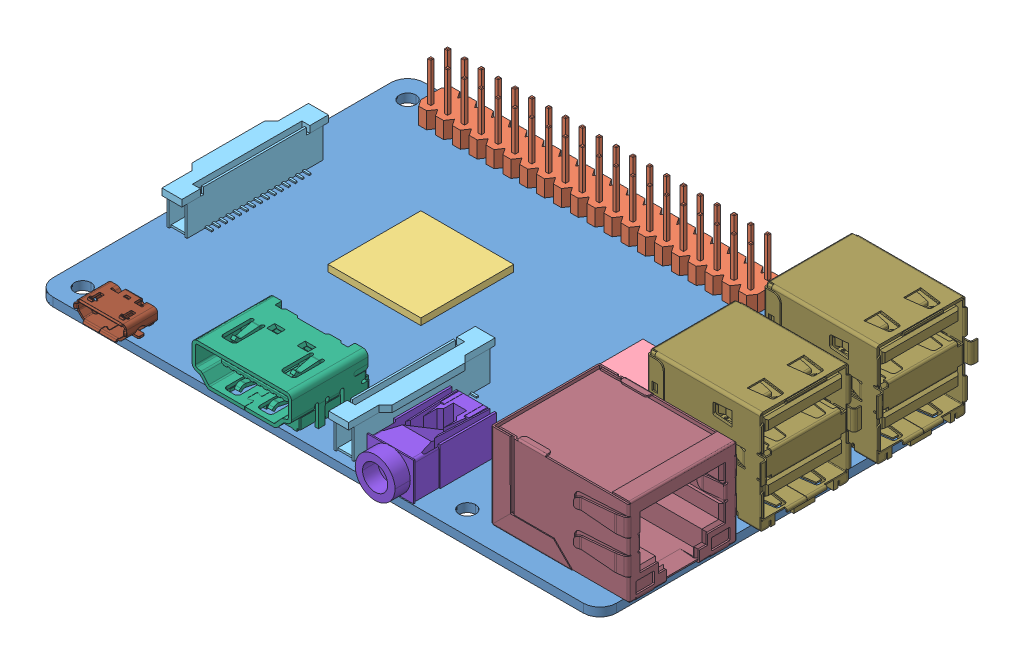
SolidWorks assembly RaspberryPi2 STEP214, configuration Default. Lengths in mm.
Overall size (89.62 18.75 58.3).
16 component instances, 13 part files, 0 mates.
Components (placement in the parent):
- RaspberryPi2 STEP214.STEP-1: RaspberryPi2 STEP214.STEP [Default] at origin size (89.62 18.75 58.3)
  - Mainboard2.STEP-1: Mainboard2.STEP [Default] at origin size (85 1.3 56)
  - GPIO.STEP-1: GPIO.STEP [Default] at (-11.37 0 -24.5) x (0 0 1) z (-1 0 0) size (5 11.5 50.8)
  - Processor.STEP-1: Processor.STEP [Default] at (-15.5 0 -3) x (0 0 1) z (-1 0 0) size (14 1 14)
  - GPU.STEP-1: GPU.STEP [Default] at (15.25 0 -5.75) x (0 0 1) z (-1 0 0) size (9.1 1 9.1)
  - CameraAssembly.STEP-1: CameraAssembly.STEP [Default] at (10.0885 -2.9159 16.55) x (-1 0 0) z (0 0 -1) size (5.01 5.51 22.11)
  - CameraAssembly.STEP-2: CameraAssembly.STEP [Default] at (-46.3885 -2.9159 0) size (5.01 5.51 22.11)
  - HDMI.STEP-1: HDMI.STEP [Default] at (-10.2 0.27 29.3) size (15.04 8.38 12.15)
  - RAM.STEP-1: RAM.STEP [Default] at (0.5 -2.3 -6) x (0 0 1) z (-1 0 0) size (12 1 12)
  - Audio.STEP-1: Audio.STEP [Default] at (10.9 0.15 21.75) size (7 6 14.8)
  - MicroSDSocket.STEP-1: MicroSDSocket.STEP [Default] at (-34.5 -1.3 -0.7) x (0 0 -1) z (-1 0 0) size (13 1.3 14)
  - MicroSD.STEP-1: MicroSD.STEP [Default] at (-37 -2.3 0.1) x (0 0 1) z (-1 0 0) size (11.01 1 15)
  - micro USB2.STEP-1: micro USB2.STEP [Default] at (-17.2704 -5.0969 44.9026) size (7.98 2.93 5.58)
  - usb double.STEP-1: usb double.STEP [Default] at (30.38 -0.09 -18.85) x (0 0 -1) z (1 0 0) size (15.6 18.75 17.92)
  - usb double.STEP-2: usb double.STEP [Default] at (30.38 -0.09 -1.25) x (0 0 -1) z (1 0 0) size (15.6 18.75 17.92)
  - RJ45-LED.STEP-1: RJ45-LED.STEP [Default] at (34.11 7.4 17.348) x (1 0 0) z (0 -1 0) size (21.3 18 14.1)
